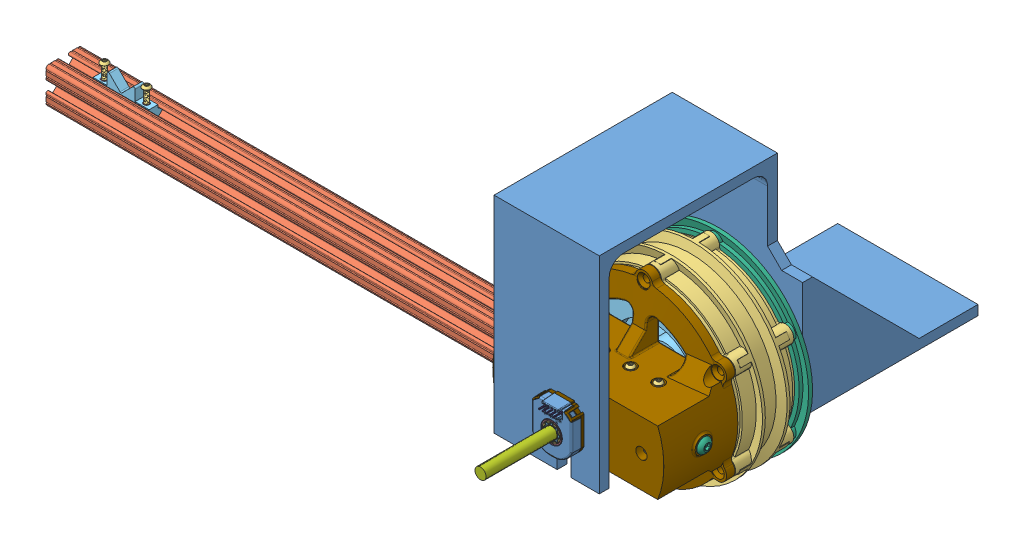
SolidWorks assembly torque_test, configuration Default. Lengths in mm.
Overall size (466.73 189.74 304.66).
83 component instances, 25 part files, 47 mates.
Components (placement in the parent):
- test_stand-2: test_stand [Default] at (3.6129 50.1777 -45.6114) size (100 147 245)
- M365 Nut-1: M365 Nut [Default] at (3.6129 80.1777 72.3886) x (1 0 0) z (0 1 0) size (23.5 10 23.5)
- M365-1: M365 [Default] at (3.6129 80.1777 115.3886) x (-0.999123 0.04186 0) z (0 0 -1) size (139.75 139.75 103.5)
  - M365 Rotor-1: M365 Rotor [Default] x (0.999123 -0.04186 0) z (0 0 1) size (134.25 134.25 41.5)
  - M365 Magnet-1: M365 Magnet [Default] at (0 0 -1.5) x (0.999123 -0.04186 0) z (0 0 1) size (11.08 3 30.5)
  - M365 Magnet-2: M365 Magnet [Default] at (0 0 -1.5) x (0.968587 -0.248675 0) z (0 0 1) size (11.08 3 30.5)
  - M365 Magnet-3: M365 Magnet [Default] at (0 0 -1.5) x (0.895719 -0.444621 0) z (0 0 1) size (11.08 3 30.5)
  - M365 Magnet-4: M365 Magnet [Default] at (0 0 -1.5) x (0.783703 -0.621136 0) z (0 0 1) size (11.08 3 30.5)
  - M365 Magnet-5: M365 Magnet [Default] at (0 0 -1.5) x (0.637436 -0.770503 0) z (0 0 1) size (11.08 3 30.5)
  - M365 Magnet-6: M365 Magnet [Default] at (0 0 -1.5) x (0.46331 -0.886196 0) z (0 0 1) size (11.08 3 30.5)
  - M365 Magnet-7: M365 Magnet [Default] at (0 0 -1.5) x (0.268935 -0.963158 0) z (0 0 1) size (11.08 3 30.5)
  - M365 Magnet-8: M365 Magnet [Default] at (0 0 -1.5) x (0.062806 -0.998026 0) z (0 0 1) size (11.08 3 30.5)
  - M365 Magnet-9: M365 Magnet [Default] at (0 0 -1.5) x (-0.146068 -0.989275 0) z (0 0 1) size (11.08 3 30.5)
  - M365 Magnet-10: M365 Magnet [Default] at (0 0 -1.5) x (-0.348558 -0.937287 0) z (0 0 1) size (11.08 3 30.5)
  - M365 Magnet-11: M365 Magnet [Default] at (0 0 -1.5) x (-0.535814 -0.844336 0) z (0 0 1) size (11.08 3 30.5)
  - M365 Magnet-12: M365 Magnet [Default] at (0 0 -1.5) x (-0.699652 -0.714484 0) z (0 0 1) size (11.08 3 30.5)
  - M365 Magnet-13: M365 Magnet [Default] at (0 0 -1.5) x (-0.832913 -0.553404 0) z (0 0 1) size (11.08 3 30.5)
  - M365 Magnet-14: M365 Magnet [Default] at (0 0 -1.5) x (-0.929771 -0.368139 0) z (0 0 1) size (11.08 3 30.5)
  - M365 Magnet-15: M365 Magnet [Default] at (0 0 -1.5) x (-0.985993 -0.166784 0) z (0 0 1) size (11.08 3 30.5)
  - M365 Magnet-16: M365 Magnet [Default] at (0 0 -1.5) x (-0.999123 0.04186 0) z (0 0 1) size (11.08 3 30.5)
  - M365 Magnet-17: M365 Magnet [Default] at (0 0 -1.5) x (-0.968587 0.248675 0) z (0 0 1) size (11.08 3 30.5)
  - M365 Magnet-18: M365 Magnet [Default] at (0 0 -1.5) x (-0.895719 0.444621 0) z (0 0 1) size (11.08 3 30.5)
  - M365 Magnet-19: M365 Magnet [Default] at (0 0 -1.5) x (-0.783703 0.621136 0) z (0 0 1) size (11.08 3 30.5)
  - M365 Magnet-20: M365 Magnet [Default] at (0 0 -1.5) x (-0.637436 0.770503 0) z (0 0 1) size (11.08 3 30.5)
  - M365 Magnet-21: M365 Magnet [Default] at (0 0 -1.5) x (-0.46331 0.886196 0) z (0 0 1) size (11.08 3 30.5)
  - M365 Magnet-22: M365 Magnet [Default] at (0 0 -1.5) x (-0.268935 0.963158 0) z (0 0 1) size (11.08 3 30.5)
  - M365 Magnet-23: M365 Magnet [Default] at (0 0 -1.5) x (-0.062806 0.998026 0) z (0 0 1) size (11.08 3 30.5)
  - M365 Magnet-24: M365 Magnet [Default] at (0 0 -1.5) x (0.146068 0.989275 0) z (0 0 1) size (11.08 3 30.5)
  - M365 Magnet-25: M365 Magnet [Default] at (0 0 -1.5) x (0.348558 0.937287 0) z (0 0 1) size (11.08 3 30.5)
  - M365 Magnet-26: M365 Magnet [Default] at (0 0 -1.5) x (0.535814 0.844336 0) z (0 0 1) size (11.08 3 30.5)
  - M365 Magnet-27: M365 Magnet [Default] at (0 0 -1.5) x (0.699652 0.714484 0) z (0 0 1) size (11.08 3 30.5)
  - M365 Magnet-28: M365 Magnet [Default] at (0 0 -1.5) x (0.832913 0.553404 0) z (0 0 1) size (11.08 3 30.5)
  - M365 Magnet-29: M365 Magnet [Default] at (0 0 -1.5) x (0.929771 0.368139 0) z (0 0 1) size (11.08 3 30.5)
  - M365 Magnet-30: M365 Magnet [Default] at (0 0 -1.5) x (0.985993 0.166784 0) z (0 0 1) size (11.08 3 30.5)
  - M365 Stator-1: M365 Stator [Default] at (0 0 -2.5) x (1 0 0) z (0 0 -1) size (105 105 103.5)
  - M365 Cap-1: M365 Cap [Default] at (0 0 21.5) x (0.999123 -0.04186 0) z (0 0 1) size (134.25 134.25 12.37)
  - 5972K83_Ball Bearing-3: 5972K83_Ball Bearing [5972K83] at (0 0 25.625) size (32 32 9)
  - 5972K83_Ball Bearing-2: 5972K83_Ball Bearing [5972K83] at (0 0 -25.25) x (1 0 0) z (0 0 -1) size (32 32 9)
  - M365 Washer-1: M365 Washer [Default] at (0 0 34.625) x (-1 0 0) z (0 -1 0) size (22 2.75 22)
- torque_test_rotor_output-1: torque_test_rotor_output [Default] at (3.6129 80.1777 136.6011) size (123 134.25 52.75)
- rotor_adaptor_ring-1: rotor_adaptor_ring [Default] at (3.6129 80.1777 137.8511) x (1 0 0) z (0 1 0) size (114.42 2.5 114.42)
- CUI_DEVICES_CUI_DEVICES_AMT103-D0048-I8000-S-1: CUI_DEVICES_CUI_DEVICES_AMT103-D0048-I8000-S [Default] at (3.6129 80.1777 203.1586) x (-1 0 0) z (0 0 1) size (36.33 37.04 14.49)
  - CUI_DEVICES_AMT-Sleeve-REV-D(8 mm)-1: CUI_DEVICES_AMT-Sleeve-REV-D(8 mm) [Default] at (0 0 -2.42) x (0.999996 0.002864 0) z (0 0 1) size (10.79 10.79 7.8)
  - CUI_DEVICES_AMT-Hub-Top-REV-D1-1: CUI_DEVICES_AMT-Hub-Top-REV-D1 [Default] at (0 0 2.13) x (0.999996 0.002864 0) z (0 0 1) size (14 14 5.67)
  - CUI_DEVICES_AMT-Hub-Bottom-REV-B-1: CUI_DEVICES_AMT-Hub-Bottom-REV-B [Default] at (0 0 2.43) x (0.999998 -0.001942 0) z (0 0 1) size (17.3 17.3 3.2)
  - CUI_DEVICES_AMT10X-Shaft-Adaptor-REV-E-1: CUI_DEVICES_AMT10X-Shaft-Adaptor-REV-E [Default] at (0 0 0.03) x (0.999996 0.002864 0) z (0 0 1) size (11.8 11.8 7.8)
  - CUI_DEVICES_Receiver-board-1: CUI_DEVICES_Receiver-board [Default] at (72.2834 -20.351 3.03) x (-1 0 0) z (0 0 -1) size (26.5 26.62 0.41)
  - CUI_DEVICES_Rotor-board-REV F-1: CUI_DEVICES_Rotor-board-REV F [Default] at (0 0 2.13) x (0.807874 -0.589355 0) z (0 0 1) size (26 26 0.3)
  - CUI_DEVICES_Transmitter-board AMT10(AMT-103)-1: CUI_DEVICES_Transmitter-board AMT10(AMT-103) [Default] at (19.1596 -17.1102 1.22) x (-1 0 0) z (0 0 -1) size (26.63 29.61 12.1)
  - CUI_DEVICES_AMT-103-Base-REV-K(Default)-1: CUI_DEVICES_AMT-103-Base-REV-K(Default) [Default] at (0 0 -1) x (-1 0 0) z (0 0 -1) size (28.59 34.62 9.11)
  - CUI_DEVICES_AMT-103-Top-Cover-REV-I-1: CUI_DEVICES_AMT-103-Top-Cover-REV-I [Default] at (0 0 5.23) x (-1 0 0) z (0 0 -1) size (28.6 33.94 9.26)
- 1010_17_48_CL-1: 1010_17_48_CL [Default] at (-390.3791 80.1277 162.1511) x (0 0 1) z (-1 0 0) size (25.4 25.4 443.99)
- 92095A472_Button Head Hex Drive Screw-1: 92095A472_Button Head Hex Drive Screw [92095A472] at (48.6129 80.1777 186.2969) size (5.7 5.7 20.01)
- 94459A140_Brass Heat-Set Inserts for Plastic-1: 94459A140_Brass Heat-Set Inserts for Plastic [94459A140] at (48.6129 80.1777 176.0511) x (1 0 0) z (0 -1 0) size (4.77 6.11 4.77)
- 92095A472_Button Head Hex Drive Screw-2: 92095A472_Button Head Hex Drive Screw [92095A472] at (18.6129 80.1777 186.2969) size (5.7 5.7 20.01)
- 92095A472_Button Head Hex Drive Screw-3: 92095A472_Button Head Hex Drive Screw [92095A472] at (-11.3871 80.1777 186.2969) size (5.7 5.7 20.01)
- 92095A472_Button Head Hex Drive Screw-4: 92095A472_Button Head Hex Drive Screw [92095A472] at (-41.3871 80.1777 186.2969) size (5.7 5.7 20.01)
- 92095A472_Button Head Hex Drive Screw-6: 92095A472_Button Head Hex Drive Screw [92095A472] at (33.6129 104.2735 162.1011) x (1 0 0) z (0 1 0) size (5.7 5.7 20.01)
- 92095A472_Button Head Hex Drive Screw-7: 92095A472_Button Head Hex Drive Screw [92095A472] at (13.6129 104.2735 162.1011) x (1 0 0) z (0 1 0) size (5.7 5.7 20.01)
- 92095A472_Button Head Hex Drive Screw-8: 92095A472_Button Head Hex Drive Screw [92095A472] at (-6.3871 104.2735 162.1011) x (1 0 0) z (0 1 0) size (5.7 5.7 20.01)
- 92095A472_Button Head Hex Drive Screw-9: 92095A472_Button Head Hex Drive Screw [92095A472] at (-26.3871 104.2735 162.1011) x (1 0 0) z (0 1 0) size (5.7 5.7 20.01)
- 92095A472_Button Head Hex Drive Screw-10: 92095A472_Button Head Hex Drive Screw [92095A472] at (33.6129 56.0819 162.1011) x (1 0 0) z (0 -1 0) size (5.7 5.7 20.01)
- 92095A472_Button Head Hex Drive Screw-11: 92095A472_Button Head Hex Drive Screw [92095A472] at (13.6129 56.0819 162.1011) x (1 0 0) z (0 -1 0) size (5.7 5.7 20.01)
- 92095A472_Button Head Hex Drive Screw-12: 92095A472_Button Head Hex Drive Screw [92095A472] at (-6.3871 56.0819 162.1011) x (1 0 0) z (0 -1 0) size (5.7 5.7 20.01)
- 92095A472_Button Head Hex Drive Screw-13: 92095A472_Button Head Hex Drive Screw [92095A472] at (-26.3871 56.0819 162.1011) x (1 0 0) z (0 -1 0) size (5.7 5.7 20.01)
- 94459A140_Brass Heat-Set Inserts for Plastic-2: 94459A140_Brass Heat-Set Inserts for Plastic [94459A140] at (33.6129 94.1777 162.1011) size (4.77 6.11 4.77)
- 94459A140_Brass Heat-Set Inserts for Plastic-3: 94459A140_Brass Heat-Set Inserts for Plastic [94459A140] at (18.6129 80.1777 176.0511) x (1 0 0) z (0 -1 0) size (4.77 6.11 4.77)
- 94459A140_Brass Heat-Set Inserts for Plastic-4: 94459A140_Brass Heat-Set Inserts for Plastic [94459A140] at (-11.3871 80.1777 176.0511) x (1 0 0) z (0 -1 0) size (4.77 6.11 4.77)
- 94459A140_Brass Heat-Set Inserts for Plastic-5: 94459A140_Brass Heat-Set Inserts for Plastic [94459A140] at (-41.3871 80.1777 176.0511) x (1 0 0) z (0 -1 0) size (4.77 6.11 4.77)
- 94459A140_Brass Heat-Set Inserts for Plastic-6: 94459A140_Brass Heat-Set Inserts for Plastic [94459A140] at (13.6129 94.1777 162.1011) size (4.77 6.11 4.77)
- 94459A140_Brass Heat-Set Inserts for Plastic-7: 94459A140_Brass Heat-Set Inserts for Plastic [94459A140] at (-6.3871 94.1777 162.1011) size (4.77 6.11 4.77)
- 94459A140_Brass Heat-Set Inserts for Plastic-8: 94459A140_Brass Heat-Set Inserts for Plastic [94459A140] at (-26.3871 94.1777 162.1011) size (4.77 6.11 4.77)
- 94459A140_Brass Heat-Set Inserts for Plastic-9: 94459A140_Brass Heat-Set Inserts for Plastic [94459A140] at (33.6129 60.4666 162.1011) size (4.77 6.11 4.77)
- 94459A140_Brass Heat-Set Inserts for Plastic-10: 94459A140_Brass Heat-Set Inserts for Plastic [94459A140] at (13.6129 60.4666 162.1011) size (4.77 6.11 4.77)
- 94459A140_Brass Heat-Set Inserts for Plastic-11: 94459A140_Brass Heat-Set Inserts for Plastic [94459A140] at (-6.3871 60.4666 162.1011) size (4.77 6.11 4.77)
- 94459A140_Brass Heat-Set Inserts for Plastic-12: 94459A140_Brass Heat-Set Inserts for Plastic [94459A140] at (-26.3871 60.4666 162.1011) size (4.77 6.11 4.77)
- rope_holder-1: rope_holder [Default] at (-346.3871 85.1179 162.1511) x (0 0 1) z (-1 0 0) size (14.5 16.34 40)
- 94459A140_Brass Heat-Set Inserts for Plastic-13: 94459A140_Brass Heat-Set Inserts for Plastic [94459A140] at (-361.3871 87.1679 162.1511) size (4.77 6.11 4.77)
- 92095A472_Button Head Hex Drive Screw-14: 92095A472_Button Head Hex Drive Screw [92095A472] at (-361.3871 104.2735 162.1511) x (1 0 0) z (0 1 0) size (5.7 5.7 20.01)
- 92095A472_Button Head Hex Drive Screw-15: 92095A472_Button Head Hex Drive Screw [92095A472] at (-331.3871 104.2735 162.1511) x (-1 0 0) z (0 1 0) size (5.7 5.7 20.01)
- 94459A140_Brass Heat-Set Inserts for Plastic-14: 94459A140_Brass Heat-Set Inserts for Plastic [94459A140] at (-331.3871 92.8791 162.1511) x (-1 0 0) z (0 0 1) size (4.77 6.11 4.77)
- 91255A818_Button Head Hex Drive Screw-1: 91255A818_Button Head Hex Drive Screw [91255A818] at (68.5339 80.1777 162.0511) x (0 0 1) z (1 0 0) size (10.41 10.41 29.08)
- shaft-1: shaft [Default] at (3.6129 80.1777 259.0511) x (1 0 0) z (0 0 -1) size (7.95 7.95 82.2)
Mates (geometry in assembly coordinates):
- Concentric1: concentric aligned: cylinder of torque_test_rotor_output-1 through (3.6129 141.1777 136.6011) axis (0 0 1) radius 2.5; cylinder of M365-1/M365 Rotor-1 through (3.6129 141.1777 130.1386) axis (0 0 1) radius 1.5
- Concentric2: concentric aligned: cylinder of torque_test_rotor_output-1 through (3.6129 19.1777 136.6011) axis (0 0 1) radius 2.5; cylinder of M365-1/M365 Rotor-1 through (3.6129 19.1777 130.1386) axis (0 0 1) radius 1.5
- Parallel15: parallel aligned: plane of M365 Nut-1 through (3.6129 80.1777 72.3886) normal (1 0 0)
- Concentric40: concentric aligned: cylinder of M365 Nut-1 through (3.6129 80.1777 62.3886) axis (0 0 1) radius 6; cylinder of M365-1/M365 Stator-1 through (3.6129 80.1777 63.6386) axis (0 0 1) radius 6
- Concentric41: concentric anti-aligned: cylinder of torque_test_rotor_output-1 through (3.6129 80.1777 142.6011) axis (0 0 -1) radius 57.2875; cylinder of rotor_adaptor_ring-1 through (3.6129 80.1777 135.3511) axis (0 0 1) radius 54.7875
- Coincident65: coincident anti-aligned: plane of torque_test_rotor_output-1 through (3.6129 80.1777 137.8511) normal (0 0 -1); plane of rotor_adaptor_ring-1 through (3.6129 80.1777 137.8511) normal (0 0 1)
- Parallel33: parallel aligned: plane of rotor_adaptor_ring-1 through (3.6129 80.1777 137.8511) normal (1 0 0)
- Coincident67: coincident aligned: cone of M365-1/M365 Rotor-1 through (3.6129 80.1777 136.1386) axis (0 0 -1); cone of rotor_adaptor_ring-1 through (3.6129 80.1777 135.3511) axis (0 0 -1)
- Parallel34: parallel anti-aligned: plane of CUI_DEVICES_CUI_DEVICES_AMT103-D0048-I8000-S-1 through (3.6129 80.1777 203.1586) normal (-1 0 0)
- Concentric44: concentric aligned: cylinder of torque_test_rotor_output-1 through (48.6129 80.1777 136.6001) axis (0 0 1) radius 1.975; cylinder of 92095A472_Button Head Hex Drive Screw-1 through (48.6129 80.1777 186.2969) axis (0 0 1) radius 2.85
- Coincident69: coincident anti-aligned: plane of torque_test_rotor_output-1 through (53.6129 67.4277 174.8511) normal (0 1 0); plane of 1010_17_48_CL-1 through (53.6129 67.4277 168.4842) normal (0 -1 0)
- Coincident70: coincident anti-aligned: plane of torque_test_rotor_output-1 through (53.6129 92.9277 174.8511) normal (0 0 -1); plane of 1010_17_48_CL-1 through (53.6129 70.5773 174.8511) normal (0 0 1)
- Parallel35: parallel aligned: plane of 3205-1 through (52.366 85.2704 172.1978) normal (1 0 0)
- Parallel36: parallel aligned: plane of 92095A472_Button Head Hex Drive Screw-1 through (48.6129 80.1777 186.2969) normal (1 0 0)
- Concentric47: concentric anti-aligned: cylinder of torque_test_rotor_output-1 through (33.6129 147.3037 162.1011) axis (0 -1 0) radius 1.975; cylinder of 92095A472_Button Head Hex Drive Screw-6 through (33.6129 104.2735 162.1011) axis (0 1 0) radius 2.85
- Parallel37: parallel aligned: plane of 92095A472_Button Head Hex Drive Screw-6 through (33.6129 104.2735 162.1011) normal (1 0 0)
- Parallel38: parallel aligned: plane of 3205-5 through (37.366 90.2869 156.9959) normal (1 0 0)
- Concentric48: concentric aligned: cylinder of M365-1/M365 Stator-1 through (3.6129 80.1777 63.6386) axis (0 0 1) radius 6; cylinder of test_stand2-1 through (3.6129 80.1777 -45.6124) axis (0 0 1) radius 6
- Coincident76: coincident anti-aligned: plane of M365 Nut-1 through (3.6129 80.1777 72.3886) normal (0 0 1); plane of test_stand2-1 through (53.6129 197.1777 72.3886) normal (0 0 -1)
- Coincident77: coincident anti-aligned: plane of M365-1/M365 Washer-1 through (3.6129 80.1777 79.3886) normal (0 0 -1); plane of test_stand-2 through (3.6129 50.1777 79.3886) normal (0 0 1)
- Coincident85: coincident anti-aligned: plane of CUI_DEVICES_CUI_DEVICES_AMT103-D0048-I8000-S-1/CUI_DEVICES_AMT-103-Base-REV-K(Default)-1 through (3.6129 80.1777 199.3886) normal (0 0 -1); plane of test_stand-2 through (3.6129 50.1777 199.3886) normal (0 0 1)
- Perpendicular1: perpendicular: plane of CUI_DEVICES_CUI_DEVICES_AMT103-D0048-I8000-S-1/CUI_DEVICES_AMT-103-Top-Cover-REV-I-1 through (17.9129 74.1978 201.8886) normal (0.999848 0 0.017452); plane of test_stand-2 through (3.6129 50.1777 -45.6114) normal (0 -1 0)
- Concentric50: concentric anti-aligned: cylinder of torque_test_rotor_output-1 through (48.6129 80.1777 136.6001) axis (0 0 1) radius 1.975; cylinder of 94459A140_Brass Heat-Set Inserts for Plastic-1 through (48.6129 80.1777 176.0511) axis (0 0 -1) radius 1.95
- Coincident86: coincident aligned: plane of torque_test_rotor_output-1 through (48.6129 80.1777 181.7511) normal (0 0 1); plane of 94459A140_Brass Heat-Set Inserts for Plastic-1 through (50.9629 80.1777 181.7511) normal (0 0 1)
- Parallel39: parallel aligned: plane of 94459A140_Brass Heat-Set Inserts for Plastic-1 through (48.6129 80.1777 176.0511) normal (1 0 0)
- Concentric51: concentric aligned: cylinder of torque_test_rotor_output-1 through (33.6129 147.3037 162.1011) axis (0 -1 0) radius 1.975; cylinder of 94459A140_Brass Heat-Set Inserts for Plastic-2 through (33.6129 94.1777 162.1011) axis (0 -1 0) radius 1.95
- Coincident88: coincident aligned: plane of torque_test_rotor_output-1 through (33.6129 99.8777 162.1011) normal (0 1 0); plane of 94459A140_Brass Heat-Set Inserts for Plastic-2 through (35.9629 99.8777 162.1011) normal (0 1 0)
- Parallel40: parallel aligned: plane of 94459A140_Brass Heat-Set Inserts for Plastic-2 through (33.6129 94.1777 162.1011) normal (1 0 0)
- Coincident90: coincident anti-aligned: plane of 1010_17_48_CL-1 through (53.6129 84.6235 163.7692) normal (0 1 0); plane of 92095A472_Button Head Hex Drive Screw-6 through (33.6129 84.6235 162.1011) normal (0 -1 0)
- Coincident91: coincident anti-aligned: plane of 1010_17_48_CL-1 through (53.6129 78.5096 166.6469) normal (0 0 1); plane of 92095A472_Button Head Hex Drive Screw-1 through (48.6129 80.1777 166.6469) normal (0 0 -1)
- Coincident92: coincident anti-aligned: plane of 1010_17_48_CL-1 through (53.6129 90.6179 155.6763) normal (0 -1 0); plane of rope_holder-1 through (-366.3871 90.6179 158.9511) normal (0 1 0)
- Width1: width anti-aligned: plane of 1010_17_48_CL-1 through (53.6129 86.4608 174.8511) normal (0 0 1); plane of rope_holder-1 through (53.6129 89.6781 149.4511) normal (0 0 -1); plane of 1010_17_48_CL-1 through (-366.3871 92.8679 158.9511) normal (0 0 -1); plane of rope_holder-1 through (-366.3871 90.6179 165.3511) normal (0 0 1)
- Distance1: distance = 350 mm anti-aligned: plane of rope_holder-1 through (-346.3871 85.1179 162.1511) normal (-1 0 0); plane of torque_test_rotor_output-1 through (3.6129 80.1777 136.6011) normal (1 0 0)
- Coincident94: coincident aligned: plane of rope_holder-1 through (-366.3871 92.8679 165.3511) normal (0 1 0); plane of 94459A140_Brass Heat-Set Inserts for Plastic-13 through (-359.0371 92.8679 162.1511) normal (0 1 0)
- Concentric52: concentric anti-aligned: cylinder of rope_holder-1 through (-361.3871 85.1179 162.1511) axis (0 1 0) radius 1.975; cylinder of 94459A140_Brass Heat-Set Inserts for Plastic-13 through (-361.3871 87.1679 162.1511) axis (0 -1 0) radius 1.95
- Parallel42: parallel aligned: plane of 94459A140_Brass Heat-Set Inserts for Plastic-13 through (-361.3871 87.1679 162.1511) normal (1 0 0)
- Concentric53: concentric aligned: cylinder of rope_holder-1 through (-361.3871 85.1179 162.1511) axis (0 1 0) radius 1.975; cylinder of 92095A472_Button Head Hex Drive Screw-14 through (-361.3871 104.2735 162.1511) axis (0 1 0) radius 2.85
- Coincident97: coincident anti-aligned: plane of 1010_17_48_CL-1 through (53.6129 84.6235 163.7692) normal (0 1 0); plane of 92095A472_Button Head Hex Drive Screw-14 through (-361.3871 84.6235 162.1511) normal (0 -1 0)
- Parallel43: parallel aligned: plane of 92095A472_Button Head Hex Drive Screw-14 through (-361.3871 104.2735 162.1511) normal (1 0 0)
- Coincident98: coincident anti-aligned: plane of torque_test_rotor_output-1 through (53.6129 80.1777 136.6011) normal (-1 0 0); plane of 1010_17_48_CL-1 through (53.6129 70.0693 149.4511) normal (1 0 0)
- Concentric54: concentric aligned: cylinder of torque_test_rotor_output-1 through (-57.3881 80.1777 162.0511) axis (1 0 0) radius 3.15; cylinder of 91255A818_Button Head Hex Drive Screw-1 through (68.5339 80.1777 162.0511) axis (1 0 0) radius 5.207
- Coincident99: coincident anti-aligned: plane of torque_test_rotor_output-1 through (65.6129 80.1777 162.0511) normal (1 0 0); plane of 91255A818_Button Head Hex Drive Screw-1 through (65.6129 85.3847 162.0511) normal (-1 0 0)
- Parallel45: parallel aligned: plane of 92949A433_18-8 Stainless Steel Button Head Hex Drive Screw-1 through (68.5339 80.1777 162.0511) normal (0 0 1)
- Coincident101: coincident anti-aligned: plane of torque_test_rotor_output-1 through (53.6129 92.9277 176.8511) normal (0 0 1); plane of shaft-1 through (3.6129 80.1777 176.8511) normal (0 0 -1)
- Concentric55: concentric aligned: cylinder of CUI_DEVICES_CUI_DEVICES_AMT103-D0048-I8000-S-1/CUI_DEVICES_AMT-Sleeve-REV-D(8 mm)-1 through (3.6129 80.1777 200.7386) axis (0 0 1) radius 4; cylinder of shaft-1 through (3.6129 80.1777 211.5511) axis (0 0 1) radius 3.975
- Width2: width anti-aligned: plane of torque_test_rotor_output-1 through (3.6129 83.6793 164.1535) normal (0 -1 0); plane of shaft-1 through (3.6129 76.6761 164.1535) normal (0 1 0); plane of torque_test_rotor_output-1 through (1.6345 83.6043 189.3511) normal (0 1 0); plane of shaft-1 through (5.5912 76.7511 189.3511) normal (0 -1 0)
- Width3: width anti-aligned: plane of torque_test_rotor_output-1 through (0.5804 81.9285 164.1535) normal (0.866025 -0.5 0); plane of shaft-1 through (6.6453 78.4269 164.1535) normal (-0.866025 0.5 0); plane of torque_test_rotor_output-1 through (-0.3438 80.1777 189.3511) normal (-0.866025 0.5 0); plane of shaft-1 through (7.5696 80.1777 189.3511) normal (0.866025 -0.5 0)
